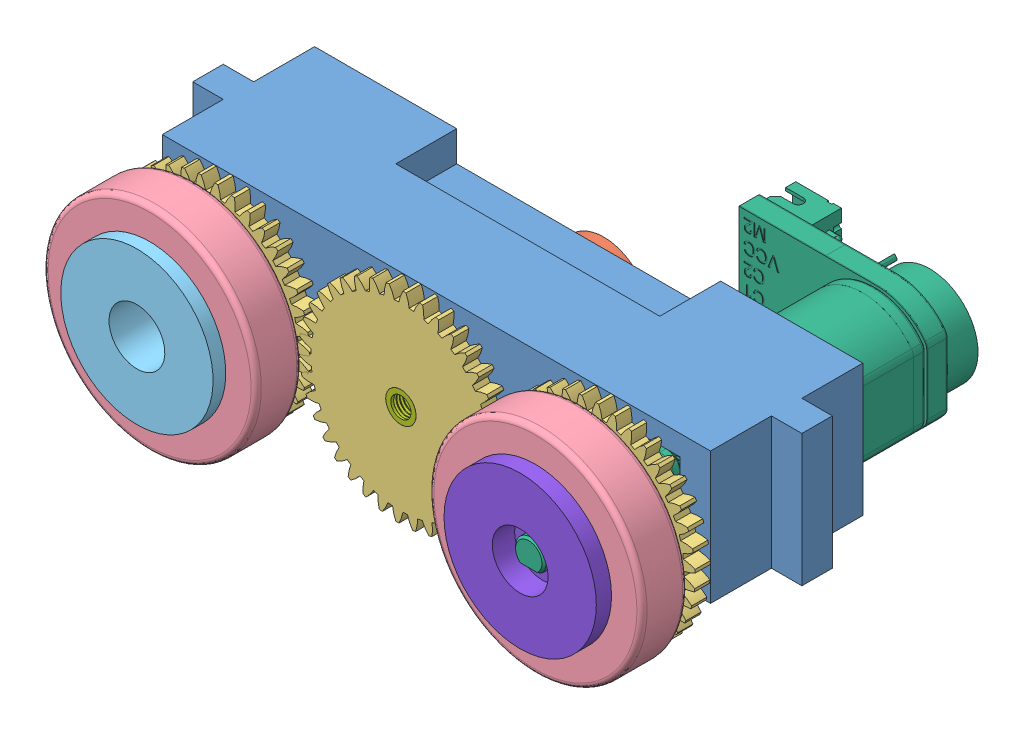
SolidWorks assembly cum banh 3.3, configuration Default. Lengths in mm.
Overall size (61.54 24.39 40.65).
15 component instances, 8 part files, 30 mates.
Components (placement in the parent):
- Ga Cum Banh 3.2-1: Ga Cum Banh 3.2 [Default] at (12.9532 31.9165 50.2873) size (60 15.5 15)
- Bac lot-1: Bac lot [Default] at (-6.0468 31.9165 59.2873) size (9 9 6)
- spur gear_iso-1: spur gear_iso [ISO - Spur gear 0.5M 38T 20PA 1.5FW ---S38A75H50L3.0N] at (12.9532 31.9165 61.2873) x (0 0 -1) z (0.998859 0.047751 0) size (1.5 19.95 20)
- Lop banh xe-1: Lop banh xe [Default] at (-6.0468 31.9165 67.7873) x (0 0 -1) z (0.984115 -0.177535 0) size (4.5 21 21)
- Mam banh xe-1: Mam banh xe [Default] at (-6.0468 31.9165 61.2873) x (-0.608419 -0.793616 0) z (0 0 -1) size (15 15 7)
- N20 Mini Micro Metall Gear Motor DC 3-6-12V-1: N20 Mini Micro Metall Gear Motor DC 3-6-12V [Default] at (31.9532 31.9165 48.6873) x (0 0 1) z (-1 0 0) size (39.8 12.15 18.58)
- spur gear_iso-2: spur gear_iso [ISO - Spur gear 0.5M 38T 20PA 1.5FW ---S38A75H50L3.0N] at (31.9532 31.9165 59.7873) x (0 0 1) z (-0.993186 0.116537 0) size (1.5 19.95 20)
- spur gear_iso-3: spur gear_iso [ISO - Spur gear 0.5M 38T 20PA 1.5FW ---S38A75H50L3.0N] at (-6.0468 31.9165 61.2873) x (0 0 -1) z (1 0 0) size (1.5 19.95 20)
- Bac lot-2: Bac lot [Default] at (12.9532 31.9165 59.2873) size (9 9 6)
- Bac lot-3: Bac lot [Default] at (12.9532 31.9165 41.2873) x (0.064602 -0.997911 0) z (0 0 -1) size (9 9 6)
- Bac lot-4: Bac lot [Default] at (-6.0468 31.9165 41.2873) x (-0.6399 -0.768458 0) z (0 0 -1) size (9 9 6)
- Tru ren trong-1: Tru ren trong [Default] at (12.9532 31.9165 61.2873) x (0.857173 -0.515029 0) z (0 0 1) size (3 3 20.11)
- Tru ren trong-2: Tru ren trong [Default] at (-6.0468 31.9165 61.2873) x (-0.86392 -0.50363 0) z (0 0 1) size (3 3 20.11)
- Lop banh xe-2: Lop banh xe [Default] at (31.9532 31.9165 67.7873) x (0 0 -1) z (-0.996477 0.083863 0) size (4.5 21 21)
- Mam banh xe 3.3-1: Mam banh xe 3.3 [Default] at (31.9532 31.9165 61.5373) x (-1 0 0) z (0 0 -1) size (15 15 7)
Mates (geometry in assembly coordinates):
- Width1: width anti-aligned: plane of N20 Mini Micro Metall Gear Motor DC 3-6-12V-1 through (36.9532 25.9165 48.6873) normal (1 0 0); plane of N20 Mini Micro Metall Gear Motor DC 3-6-12V-1 through (26.9532 37.9165 48.6873) normal (-1 0 0); plane of Ga Cum Banh 3.2-1 through (36.9532 31.9165 57.7873) normal (-1 0 0); plane of Ga Cum Banh 3.2-1 through (26.9532 31.9165 57.7873) normal (1 0 0)
- Coincident1: coincident anti-aligned: plane of Ga Cum Banh 3.2-1 through (12.9532 37.9165 57.7873) normal (0 -1 0); plane of N20 Mini Micro Metall Gear Motor DC 3-6-12V-1 through (36.9532 37.9165 52.7873) normal (0 1 0)
- Concentric1: concentric anti-aligned: cylinder of Ga Cum Banh 3.2-1 through (-6.0468 31.9165 57.7873) axis (0 0 -1) radius 3.15; cylinder of spur gear_iso-3 through (-6.0468 31.9165 11.2872) axis (0 0 1) radius 1.5
- Concentric2: concentric anti-aligned: cylinder of N20 Mini Micro Metall Gear Motor DC 3-6-12V-1 through (31.9532 31.9165 67.6873) axis (0 0 1) radius 1.5; cylinder of spur gear_iso-2 through (31.9532 31.9165 109.7873) axis (0 0 -1) radius 1.5
- Concentric3: concentric anti-aligned: cylinder of Ga Cum Banh 3.2-1 through (12.9532 31.9165 57.7873) axis (0 0 -1) radius 3.15; cylinder of spur gear_iso-1 through (12.9532 31.9165 11.2872) axis (0 0 1) radius 1.5
- Coincident2: coincident aligned: plane of spur gear_iso-1 through (12.9532 31.9165 59.7873) normal (0 0 -1); plane of spur gear_iso-2 through (31.9532 31.9165 59.7873) normal (0 0 -1)
- Coincident3: coincident aligned: plane of spur gear_iso-1 through (12.9532 31.9165 59.7873) normal (0 0 -1); plane of spur gear_iso-3 through (-6.0468 31.9165 59.7873) normal (0 0 -1)
- Concentric4: concentric anti-aligned: cylinder of Ga Cum Banh 3.2-1 through (-6.0468 31.9165 57.7873) axis (0 0 -1) radius 3.15; cylinder of Bac lot-1 through (-6.0468 31.9165 59.2873) axis (0 0 1) radius 3
- Coincident4: coincident anti-aligned: plane of Ga Cum Banh 3.2-1 through (12.9532 31.9165 57.7873) normal (0 0 1); plane of Bac lot-1 through (-3.0468 31.9165 57.7873) normal (0 0 -1)
- Concentric5: concentric aligned: cylinder of Ga Cum Banh 3.2-1 through (-6.0468 31.9165 57.7873) axis (0 0 -1) radius 3.15; cylinder of Bac lot-4 through (-6.0468 31.9165 41.2873) axis (0 0 -1) radius 3
- Coincident5: coincident anti-aligned: plane of Ga Cum Banh 3.2-1 through (12.9532 31.9165 42.7873) normal (0 0 -1); plane of Bac lot-4 through (-7.9665 29.6112 42.7873) normal (0 0 1)
- Concentric6: concentric anti-aligned: cylinder of Ga Cum Banh 3.2-1 through (12.9532 31.9165 57.7873) axis (0 0 -1) radius 3.15; cylinder of Bac lot-2 through (12.9532 31.9165 59.2873) axis (0 0 1) radius 3
- Coincident6: coincident anti-aligned: plane of Ga Cum Banh 3.2-1 through (12.9532 31.9165 57.7873) normal (0 0 1); plane of Bac lot-2 through (15.9532 31.9165 57.7873) normal (0 0 -1)
- Concentric7: concentric aligned: cylinder of Ga Cum Banh 3.2-1 through (12.9532 31.9165 57.7873) axis (0 0 -1) radius 3.15; cylinder of Bac lot-3 through (12.9532 31.9165 41.2873) axis (0 0 -1) radius 3
- Coincident7: coincident anti-aligned: plane of Ga Cum Banh 3.2-1 through (12.9532 31.9165 42.7873) normal (0 0 -1); plane of Bac lot-3 through (13.147 28.9228 42.7873) normal (0 0 1)
- Distance1: distance = 0.5 mm anti-aligned: plane of spur gear_iso-1 through (12.9532 31.9165 59.7873) normal (0 0 -1); plane of Bac lot-2 through (17.4532 31.9165 59.2873) normal (0 0 1)
- Distance2: distance = 0.5 mm anti-aligned: plane of spur gear_iso-2 through (31.9532 31.9165 59.7873) normal (0 0 -1); plane of N20 Mini Micro Metall Gear Motor DC 3-6-12V-1 through (34.4532 29.4165 59.2873) normal (0 0 1)
- Concentric8: concentric anti-aligned: cylinder of Bac lot-4 through (-6.0468 31.9165 41.2873) axis (0 0 -1) radius 1.65; cylinder of Tru ren trong-2 through (-6.0468 31.9165 61.2873) axis (0 0 1) radius 1.5
- Concentric9: concentric aligned: cylinder of spur gear_iso-1 through (12.9532 31.9165 11.2872) axis (0 0 1) radius 1.5; cylinder of Tru ren trong-1 through (12.9532 31.9165 61.2873) axis (0 0 1) radius 1.5
- Concentric10: concentric anti-aligned: cylinder of Lop banh xe-1 through (-6.0468 31.9165 67.7873) axis (0 0 1) radius 5.5; cylinder of Mam banh xe-1 through (-6.0468 31.9165 61.2873) axis (0 0 -1) radius 5.5
- Coincident10: coincident anti-aligned: plane of Lop banh xe-1 through (-4.1827 42.2497 62.5373) normal (0 0 -1); plane of Mam banh xe-1 through (-10.61 25.9644 62.5373) normal (0 0 1)
- Coincident15: coincident anti-aligned: plane of Mam banh xe-1 through (-7.0507 30.6071 61.2873) normal (0 0 -1); plane of spur gear_iso-3 through (-6.0468 31.9165 61.2873) normal (0 0 1)
- Coincident17: coincident aligned: plane of spur gear_iso-1 through (12.9532 31.9165 61.2873) normal (0 0 1); plane of Tru ren trong-1 through (13.8104 31.4015 61.2873) normal (0 0 1)
- Coincident18: coincident aligned: plane of Bac lot-4 through (-8.9264 28.4585 41.2873) normal (0 0 -1); plane of Tru ren trong-2 through (-7.3427 31.1611 41.2873) normal (0 0 -1)
- Concentric15: concentric anti-aligned: cylinder of Mam banh xe-1 through (-6.0468 31.9165 61.2873) axis (0 0 -1) radius 1.65; circle of Tru ren trong-2
- Concentric16: concentric aligned: cylinder of N20 Mini Micro Metall Gear Motor DC 3-6-12V-1 through (31.9532 31.9165 67.6873) axis (0 0 1) radius 1.5; cylinder of Mam banh xe 3.3-1 through (31.9532 31.9165 58.5373) axis (0 0 1) radius 1.6
- Coincident19: coincident anti-aligned: plane of Lop banh xe-2 through (31.0726 21.4535 62.5373) normal (0 0 -1); plane of Mam banh xe 3.3-1 through (24.4532 31.9165 62.5373) normal (0 0 1)
- Coincident20: coincident aligned: plane of Lop banh xe-1 through (-4.1827 42.2497 62.5373) normal (0 0 -1); plane of Lop banh xe-2 through (31.0726 21.4535 62.5373) normal (0 0 -1)
- Concentric17: concentric anti-aligned: cylinder of Lop banh xe-2 through (31.9532 31.9165 67.7873) axis (0 0 1) radius 5.5; cylinder of Mam banh xe 3.3-1 through (31.9532 31.9165 61.5373) axis (0 0 -1) radius 5.5
- Parallel1: parallel anti-aligned: plane of N20 Mini Micro Metall Gear Motor DC 3-6-12V-1 through (33.9532 30.9165 59.6873) normal (0 -1 0); plane of Mam banh xe 3.3-1 through (30.7913 30.8165 61.5373) normal (0 1 0)
